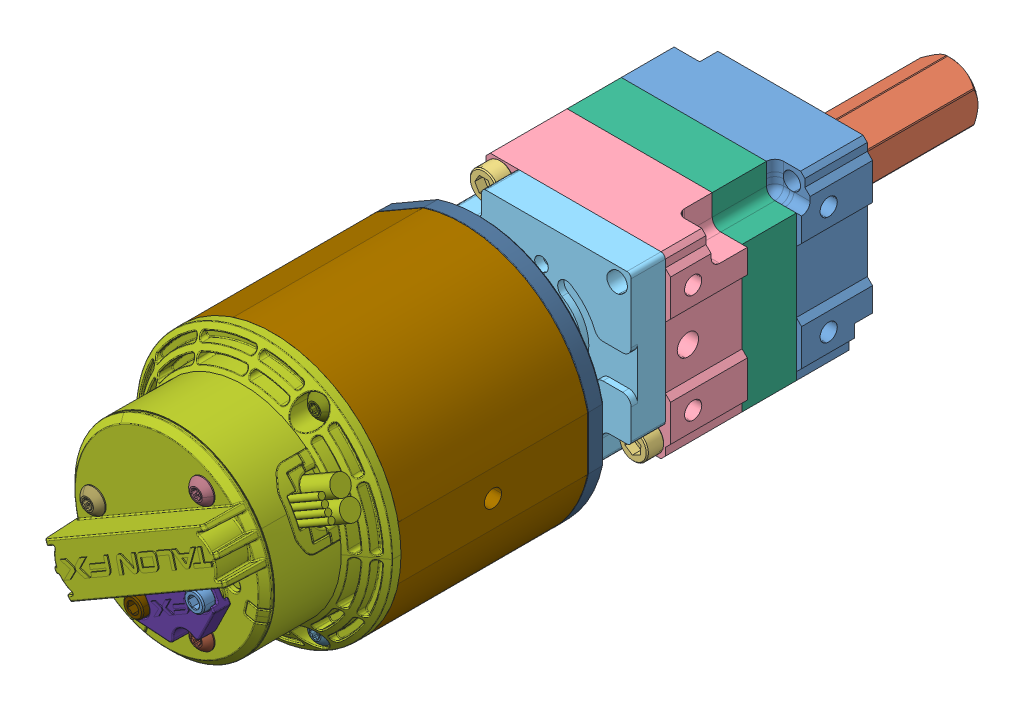
SolidWorks assembly MotorStack, configuration Default. Lengths in mm.
Overall size (81.62 81.39 192.35).
31 component instances, 25 part files, 2 mates.
Components (placement in the parent):
- v2-VersaPlanetary-1stage-with-AM9015-20131031-1: v2-VersaPlanetary-1stage-with-AM9015-20131031 [Default] at (32.9453 91.261 18.2063) x (0 0 -1) z (0 1 0) size (95.9 44.45 42.1)
  - 217-2625-026 Rev1-1: 217-2625-026 Rev1 [Default] at (-6.5 22.225 0) x (0 -1 0) z (-1 0 0) size (44.45 42 18.13)
  - 217-2742-001 Rev4-1: 217-2742-001 Rev4 [Default] at (0.2002 22.225 0) x (1 0 0) z (0 -0.092627 0.995701) size (7 28 28)
  - 217-2742-001 Rev4-2: 217-2742-001 Rev4 [Default] at (8.2002 22.225 0) size (7 28 28)
  - 217-2625-017 Rev1_9714K61-1: 217-2625-017 Rev1_9714K61 [Default] at (7.42 22.3002 -0.342) x (0 0.56703 0.823697) z (0 -0.823697 0.56703) size (28.51 4.98 30.18)
  - 217-2625-003 Rev1-1: 217-2625-003 Rev1 [Default] at (7.4478 22.225 0) x (0 -1 0) z (1 0 0) size (17 17 64.12)
  - 217-2625-018 Rev1_98541A410-1: 217-2625-018 Rev1_98541A410 [Default] at (-0.7046 22.225 0) x (1 0 0) z (0 -0.017452 0.999848) size (1 19.6 17.4)
  - 832-1750-Ring-Gear-Screw_SSA0832-0500ZC-1: 832-1750-Ring-Gear-Screw_SSA0832-0500ZC [Default] at (-30.7 4.725 -17.5) x (0 0.997447 0.071411) z (0 -0.071411 0.997447) size (6.73 48.51 6.73)
  - 832-1750-Ring-Gear-Screw_SSA0832-0500ZC-2: 832-1750-Ring-Gear-Screw_SSA0832-0500ZC [Default] at (-30.7 39.725 17.5) x (0 0.005929 0.999982) z (0 -0.999982 0.005929) size (6.73 48.51 6.73)
  - 217-2625-025 Rev1-1: 217-2625-025 Rev1 [Default] at (-23.2 22.225 0) x (0 -1 0) z (-1 0 0) size (44.45 42 18)
  - 217-2822-004 Rev4-1: 217-2822-004 Rev4 [Default] at (-37.7 22.225 0) x (0 -1 0) z (-1 0 0) size (42 42 9.8)
  - 217-2820 Rev1_Public-1: 217-2820 Rev1_Public [Default] at (-4.6546 22.225 0) x (0 -0.456494 0.889726) z (-1 0 0)
    - 217-2625-100-1: 217-2625-100 [Default] at origin
  - 217-2816-001 Rev1-1: 217-2816-001 Rev1 [Default] at (-6.35 22.225 0) x (0 -1 0) z (1 0 0) size (42 42 14.5)
  - 217-4649-001 Rev1-1: 217-4649-001 Rev1 [Default] at (-20.046 22.225 0) x (0 -1 0) z (1 0 0) size (18 18 13)
  - 217-4649-007 Rev1_94105A824-1: 217-4649-007 Rev1_94105A824 [Default] at (-25.521 22.225 -6.7835) x (-0.996104 -0.088191 0) z (0 0 -1) size (4.83 4.83 4.9)
  - 217-2625-014 Rev2-1: 217-2625-014 Rev2 [Default] at (-24.7818 22.225 0) x (0 0 1) z (0 -1 0) size (8.01 7.5 7.94)
- Falcon_500_Powered_by_Talon_FX_217-6515-1: Falcon_500_Powered_by_Talon_FX_217-6515 [Default] at (9.4877 97.4968 108.3478) x (1 0 0) z (0 0 -1) size (81.62 81.39 116.76)
  - Copy of 217-6515-Back 20190920^Falcon_500_Powered_by_Talon_FX_217-6515-1: Copy of 217-6515-Back 20190920^Falcon_500_Powered_by_Talon_FX_217-6515 [Default] at (1.2326 6.2358 -14.9619) size (60.06 60.12 79.55) (virtual)
  - Copy of Copy of 217-6515-201 Rev6^Falcon_500_Powered_by_Talon_FX_217-6515-1: Copy of Copy of 217-6515-201 Rev6^Falcon_500_Powered_by_Talon_FX_217-6515 [Default] at (1.2326 6.2358 50.6381) x (0.809017 0.587785 0) z (0 0 1) size (9.31 9.33 42.21) (virtual)
  - Copy of 217-6515-002 Rev6^Falcon_500_Powered_by_Talon_FX_217-6515-1: Copy of 217-6515-002 Rev6^Falcon_500_Powered_by_Talon_FX_217-6515 [Default] at (1.2326 6.2358 10.7381) x (0 -1 0) z (0 0 1) size (60 59.34 44.4) (virtual)
  - Copy of 217-6515-001 Rev6^Falcon_500_Powered_by_Talon_FX_217-6515-1: Copy of 217-6515-001 Rev6^Falcon_500_Powered_by_Talon_FX_217-6515 [Default] at (1.2326 6.2358 30.9381) x (0.5 0.866025 0) z (0 0 1) size (59.34 59.99 10) (virtual)
  - Copy of M3 BHTS-SECURE, Grade 8 Steel Rev1_SBTM3-24MMZB-SECURE^Falcon_500_Powered_by_Talon_FX_217-6515-1: Copy of M3 BHTS-SECURE, Grade 8 Steel Rev1_SBTM3-24MMZB-SECURE^Falcon_500_Powered_by_Talon_FX_217-6515 [Default] at (9.7324 20.9581 -38.0119) x (-0.923728 -0.383049 0) z (0 0 -1) size (5.69 5.69 25.65) (virtual)
  - Copy (2) of M3 BHTS-SECURE, Grade 8 Steel Rev1_SBTM3-24MMZB-SECURE^Falcon_500_Powered_by_Talon_FX_217-6515-2: Copy (2) of M3 BHTS-SECURE, Grade 8 Steel Rev1_SBTM3-24MMZB-SECURE^Falcon_500_Powered_by_Talon_FX_217-6515 [Default] at (-15.7672 6.2357 -38.0119) x (0.793594 -0.608447 0) z (0 0 -1) size (5.69 5.69 25.65) (virtual)
  - Copy (3) of M3 BHTS-SECURE, Grade 8 Steel Rev1_SBTM3-24MMZB-SECURE^Falcon_500_Powered_by_Talon_FX_217-6515-3: Copy (3) of M3 BHTS-SECURE, Grade 8 Steel Rev1_SBTM3-24MMZB-SECURE^Falcon_500_Powered_by_Talon_FX_217-6515 [Default] at (9.7326 -8.4864 -38.0119) x (0.130134 0.991496 0) z (0 0 -1) size (5.69 5.69 25.65) (virtual)
  - Copy of M3 BHTS, Grade 8 Steel Rev1_SBTM3-50MMZB^Falcon_500_Powered_by_Talon_FX_217-6515-1: Copy of M3 BHTS, Grade 8 Steel Rev1_SBTM3-50MMZB^Falcon_500_Powered_by_Talon_FX_217-6515 [Default] at (14.3576 28.969 -14.8619) x (-0.923728 -0.383049 0) z (0 0 -1) size (5.7 5.7 51.65) (virtual)
  - Copy (2) of M3 BHTS, Grade 8 Steel Rev1_SBTM3-50MMZB^Falcon_500_Powered_by_Talon_FX_217-6515-2: Copy (2) of M3 BHTS, Grade 8 Steel Rev1_SBTM3-50MMZB^Falcon_500_Powered_by_Talon_FX_217-6515 [Default] at (-25.0174 6.2358 -14.8619) x (0.793594 -0.608447 0) z (0 0 -1) size (5.7 5.7 51.65) (virtual)
  - Copy (3) of M3 BHTS, Grade 8 Steel Rev1_SBTM3-50MMZB^Falcon_500_Powered_by_Talon_FX_217-6515-3: Copy (3) of M3 BHTS, Grade 8 Steel Rev1_SBTM3-50MMZB^Falcon_500_Powered_by_Talon_FX_217-6515 [Default] at (14.3576 -16.4974 -14.8619) x (0.130134 0.991496 0) z (0 0 -1) size (5.7 5.7 51.65) (virtual)
  - Copy of 217-6515-308 Rev5^Falcon_500_Powered_by_Talon_FX_217-6515-1: Copy of 217-6515-308 Rev5^Falcon_500_Powered_by_Talon_FX_217-6515 [Default] at (7.0724 16.3512 -38.3619) x (0.866013 -0.500022 0) z (0.500022 0.866013 0) size (21.32 4.25 9.95) (virtual)
  - Copy of #4-40 SHCS, Grade 8 Steel Rev2_SSA0440-0125ZB^Falcon_500_Powered_by_Talon_FX_217-6515-1: Copy of #4-40 SHCS, Grade 8 Steel Rev2_SSA0440-0125ZB^Falcon_500_Powered_by_Talon_FX_217-6515 [Default] at (-1.3722 18.2247 -35.6869) x (-0.90374 0.428082 0) z (0 0 -1) size (4.65 4.65 6.03) (virtual)
  - Copy (2) of #4-40 SHCS, Grade 8 Steel Rev2_SSA0440-0125ZB^Falcon_500_Powered_by_Talon_FX_217-6515-2: Copy (2) of #4-40 SHCS, Grade 8 Steel Rev2_SSA0440-0125ZB^Falcon_500_Powered_by_Talon_FX_217-6515 [Default] at (12.917 9.9744 -35.6869) x (-0.992189 0.124742 0) z (0 0 -1) size (4.65 4.65 6.03) (virtual)
Mates (geometry in assembly coordinates):
- Concentric1: concentric aligned: cylinder of v2-VersaPlanetary-1stage-with-AM9015-20131031-1/217-2822-004 Rev4-1 through (10.7203 91.261 56.9063) axis (0 0 -1) radius 6.5; cone of Falcon_500_Powered_by_Talon_FX_217-6515-1/Falcon_500_Powered_by_Talon_FX_217-6515(2)^Falcon_500_Powered_by_Talon_FX_217-6515-1/217-6515-001 Rev6^Falcon_500_Powered_by_Talon_FX_217-6515(2)_Falcon_500_Powered_by_Talon_FX_217-6515-1 through (10.7203 91.261 71.4097) axis (0 0 -1)
- Distance1: distance = 14.5034 mm anti-aligned: plane of Falcon_500_Powered_by_Talon_FX_217-6515-1/Falcon_500_Powered_by_Talon_FX_217-6515(2)^Falcon_500_Powered_by_Talon_FX_217-6515-1/217-6515-001 Rev6^Falcon_500_Powered_by_Talon_FX_217-6515(2)_Falcon_500_Powered_by_Talon_FX_217-6515-1 through (5.9578 99.5099 71.4097) normal (0 0 -1); plane of v2-VersaPlanetary-1stage-with-AM9015-20131031-1/217-2822-004 Rev4-1 through (10.7203 91.261 56.9063) normal (0 0 1)
